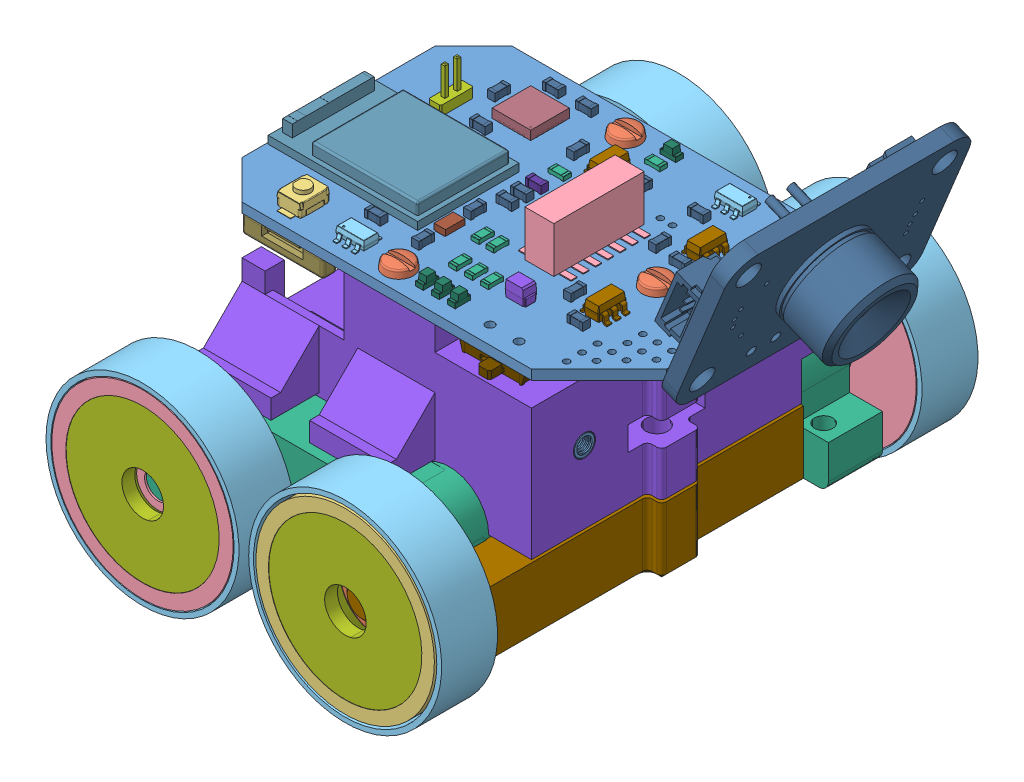
SolidWorks assembly AstroAnt_small_magnet, configuration Default. Lengths in mm.
Overall size (60.89 48.29 55.6).
184 component instances, 52 part files, 56 mates.
Components (placement in the parent):
- LiPo_360mAh-1: LiPo_360mAh [Default] at (6.0099 4.9998 47.0256) size (26.5 4.2 23.5) (hidden)
- 92120A150_Brass Heat-Set Inserts for Plastic-1: 92120A150_Brass Heat-Set Inserts for Plastic [92120A150] at (19.9543 12.4998 45.7029) size (2.56 3.33 2.56)
- 92120A150_Brass Heat-Set Inserts for Plastic-2: 92120A150_Brass Heat-Set Inserts for Plastic [92120A150] at (4.9543 12.4998 33.9529) size (2.56 3.33 2.56)
- 92120A150_Brass Heat-Set Inserts for Plastic-3: 92120A150_Brass Heat-Set Inserts for Plastic [92120A150] at (4.9543 12.4998 57.4529) size (2.56 3.33 2.56)
- 91460A005_METRIC CHEESE HEAD SLOTTED MACHINE SCREW-8: 91460A005_METRIC CHEESE HEAD SLOTTED MACHINE SCREW [91460A005] at (4.9543 14.9998 57.4529) x (1 0 0) z (0 1 0) size (3 3 7.1)
- 91460A005_METRIC CHEESE HEAD SLOTTED MACHINE SCREW-9: 91460A005_METRIC CHEESE HEAD SLOTTED MACHINE SCREW [91460A005] at (4.9543 14.9998 33.9529) x (1 0 0) z (0 1 0) size (3 3 7.1)
- 91460A005_METRIC CHEESE HEAD SLOTTED MACHINE SCREW-10: 91460A005_METRIC CHEESE HEAD SLOTTED MACHINE SCREW [91460A005] at (19.9543 14.9998 45.7029) x (1 0 0) z (0 1 0) size (3 3 7.1)
- 92120A150_Brass Heat-Set Inserts for Plastic-4: 92120A150_Brass Heat-Set Inserts for Plastic [92120A150] at (4.9543 -0.6002 57.4529) x (-0.616962 0 -0.786993) z (0.786993 0 -0.616962) size (2.56 3.33 2.56)
- 92120A150_Brass Heat-Set Inserts for Plastic-5: 92120A150_Brass Heat-Set Inserts for Plastic [92120A150] at (4.9543 -0.6002 33.9529) x (-0.616962 0 -0.786993) z (0.786993 0 -0.616962) size (2.56 3.33 2.56)
- mainboard_v1.step-1: mainboard_v1.step [Default] at (-103.0457 13.9998 235.7029) x (0 0 -1) z (0 1 0) size (29.41 41 10.8)
  - B3U-1000P.step-1: B3U-1000P.step [Default] at (178.95 -97.38 1.05) x (1 0 0) z (0 -1 0) size (4 1.75 2.5)
    - COMPOUND.step-1: COMPOUND.step [Default] at origin size (4 1.75 2.5)
  - 20021321-00014C1LF.step-1: 20021321-00014C1LF.step [Default] at (190 -115.5 1.05) size (9.35 5.45 4.85)
    - COMPOUND-0.step-1: COMPOUND-0.step [Default] at origin size (9.35 5.45 4.85)
  - MP6513GJ-Z.step-1: MP6513GJ-Z.step [Default] at (201.21 -120 1.05) x (-1 0 0) z (0 0 1) size (2.8 2.9 1)
    - COMPOUND-1.step-1: COMPOUND-1.step [Default] at origin size (2.8 2.9 1)
  - MP6513GJ-Z.step-2: MP6513GJ-Z.step [Default] at (178.51 -103.46 1.05) size (2.8 2.9 1)
    - COMPOUND-1.step-1: COMPOUND-1.step [Default] at origin size (2.8 2.9 1)
  - R_0603_1608Metric.step-1: R_0603_1608Metric.step [Default] at (195.55 -104.38 -0.05) x (1 0 0) z (0 0 -1) size (1.6 0.8 0.45)
    - SOLID.step-1: SOLID.step [Default] at origin size (1.6 0.8 0.45)
  - R_0603_1608Metric.step-2: R_0603_1608Metric.step [Default] at (192.6 -99.86 -0.05) x (0 1 0) z (0 0 -1) size (1.6 0.8 0.45)
    - SOLID.step-1: SOLID.step [Default] at origin size (1.6 0.8 0.45)
  - PinHeader_2x01_P1.27mm_Vertical.step-1: PinHeader_2x01_P1.27mm_Vertical.step [Default] at (194.96 -96.07 1.05) size (3.4 1.27 6.3)
    - SOLID-2.step-1: SOLID-2.step [Default] at origin size (3.4 1.27 6.3)
  - TAJP106K010RNJ.step-1: TAJP106K010RNJ.step [Default] at (196.22 -98.14 -0.05) x (-1 0 0) z (0 0 -1) size (2.05 1.4 1.7)
    - COMPOUND-3.step-1: COMPOUND-3.step [Default] at origin size (2.05 1.4 1.7)
  - TAJP106K010RNJ.step-2: TAJP106K010RNJ.step [Default] at (181.68 -117.23 1.05) x (0 1 0) z (0 0 1) size (2.05 1.4 1.7)
    - COMPOUND-3.step-1: COMPOUND-3.step [Default] at origin size (2.05 1.4 1.7)
  - SOT-23-5.step-1: SOT-23-5.step [Default] at (195.38 -122.78 1.05) x (0 1 0) z (0 0 1) size (2.8 2.9 1.55)
    - SOLID-4.step-1: SOLID-4.step [Default] at origin size (2.8 2.9 1.55)
  - C_0603_1608Metric.step-1: C_0603_1608Metric.step [Default] at (192.91 -122.55 1.05) x (0 -1 0) z (0 0 1) size (1.6 0.8 0.8)
    - SOLID-5.step-1: SOLID-5.step [Default] at origin size (1.6 0.8 0.8)
  - C_0603_1608Metric.step-2: C_0603_1608Metric.step [Default] at (193.57 -119.76 1.05) size (1.6 0.8 0.8)
    - SOLID-5.step-1: SOLID-5.step [Default] at origin size (1.6 0.8 0.8)
  - ECS-.327-12.5-12-TR.step-1: ECS-.327-12.5-12-TR.step [Default] at (184.31 -107.18 1.05) size (2 1.2 0.7)
    - COMPOUND-6.step-1: COMPOUND-6.step [Default] at origin size (2 1.2 0.7)
  - C_0603_1608Metric.step-3: C_0603_1608Metric.step [Default] at (197.67 -113.69 1.05) size (1.6 0.8 0.8)
    - SOLID-5.step-1: SOLID-5.step [Default] at origin size (1.6 0.8 0.8)
  - C_0603_1608Metric.step-4: C_0603_1608Metric.step [Default] at (197.64 -107.18 1.05) size (1.6 0.8 0.8)
    - SOLID-5.step-1: SOLID-5.step [Default] at origin size (1.6 0.8 0.8)
  - C_0603_1608Metric.step-5: C_0603_1608Metric.step [Default] at (190.96 -108.09 1.05) x (0 1 0) z (0 0 1) size (1.6 0.8 0.8)
    - SOLID-5.step-1: SOLID-5.step [Default] at origin size (1.6 0.8 0.8)
  - 1734592-6.step-1: 1734592-6.step [Default] at (203.79 -118 -1.05) x (0 -1 0) z (1 0 0) size (8.43 2.05 5.11)
    - SOLID-7.step-1: SOLID-7.step [Default] at origin size (8.43 2.05 5.11)
  - 1734592-6.step-2: 1734592-6.step [Default] at (176.19 -98 -1.05) x (0 1 0) z (-1 0 0) size (8.43 2.05 5.11)
    - SOLID-7.step-1: SOLID-7.step [Default] at origin size (8.43 2.05 5.11)
  - 20021321-00010C4LF.step-1: 20021321-00010C4LF.step [Default] at (190 -127.85 -0.05) x (1 0 0) z (0 0 -1) size (6.81 5.45 4.85)
    - COMPOUND-8.step-1: COMPOUND-8.step [Default] at origin size (6.81 5.45 4.85) (hidden)
  - 20021321-00010C4LF.step-2: 20021321-00010C4LF.step [Default] at (190 -127.85 1.05) size (6.81 5.45 4.85)
    - COMPOUND-8.step-1: COMPOUND-8.step [Default] at origin size (6.81 5.45 4.85) (hidden)
  - C_0603_1608Metric.step-6: C_0603_1608Metric.step [Default] at (181.31 -102.6 1.05) x (0 -1 0) z (0 0 1) size (1.6 0.8 0.8)
    - SOLID-5.step-1: SOLID-5.step [Default] at origin size (1.6 0.8 0.8)
  - C_0603_1608Metric.step-7: C_0603_1608Metric.step [Default] at (198.25 -119.14 1.05) x (0 -1 0) z (0 0 1) size (1.6 0.8 0.8)
    - SOLID-5.step-1: SOLID-5.step [Default] at origin size (1.6 0.8 0.8)
  - MPU6050.step-1: MPU6050.step [Default] at (198.43 -101.5 1.05) x (0 1 0) z (1 0 0) size (4 0.95 4)
    - COMPOUND-9.step-1: COMPOUND-9.step [Default] at origin size (4 0.95 4)
  - C_0603_1608Metric.step-8: C_0603_1608Metric.step [Default] at (194.9 -99.89 1.05) x (0 -1 0) z (0 0 1) size (1.6 0.8 0.8)
    - SOLID-5.step-1: SOLID-5.step [Default] at origin size (1.6 0.8 0.8)
  - C_0603_1608Metric.step-9: C_0603_1608Metric.step [Default] at (201.98 -100.38 1.05) x (0 -1 0) z (0 0 1) size (1.6 0.8 0.8)
    - SOLID-5.step-1: SOLID-5.step [Default] at origin size (1.6 0.8 0.8)
  - C_0603_1608Metric.step-10: C_0603_1608Metric.step [Default] at (201.98 -103.78 1.05) x (0 1 0) z (0 0 1) size (1.6 0.8 0.8)
    - SOLID-5.step-1: SOLID-5.step [Default] at origin size (1.6 0.8 0.8)
  - C_0603_1608Metric.step-11: C_0603_1608Metric.step [Default] at (198.81 -97.82 1.05) size (1.6 0.8 0.8)
    - SOLID-5.step-1: SOLID-5.step [Default] at origin size (1.6 0.8 0.8)
  - SOT-23-5.step-2: SOT-23-5.step [Default] at (184.86 -122.77 1.05) x (0 1 0) z (0 0 1) size (2.8 2.9 1.55)
    - SOLID-4.step-1: SOLID-4.step [Default] at origin size (2.8 2.9 1.55)
  - SOT-23-5.step-3: SOT-23-5.step [Default] at (197.58 -110.46 1.05) x (0 1 0) z (0 0 1) size (2.8 2.9 1.55)
    - SOLID-4.step-1: SOLID-4.step [Default] at origin size (2.8 2.9 1.55)
  - MDBT50Q-1MV2.step-1: MDBT50Q-1MV2.step [Default] at (187.3136 -98.605 1.0754) x (-1 0 0) z (0 1 0) size (10.5 2.06 15.5)
    - SOLID-10.step-1: SOLID-10.step [Default] at origin size (10.5 2.06 15.5)
  - C_0603_1608Metric.step-12: C_0603_1608Metric.step [Default] at (189.44 -108.09 1.05) x (0 1 0) z (0 0 1) size (1.6 0.8 0.8)
    - SOLID-5.step-1: SOLID-5.step [Default] at origin size (1.6 0.8 0.8)
  - C_0603_1608Metric.step-13: C_0603_1608Metric.step [Default] at (181.57 -107.18 1.05) x (-1 0 0) z (0 0 1) size (1.6 0.8 0.8)
    - SOLID-5.step-1: SOLID-5.step [Default] at origin size (1.6 0.8 0.8)
  - C_0603_1608Metric.step-14: C_0603_1608Metric.step [Default] at (186.97 -107.18 1.05) size (1.6 0.8 0.8)
    - SOLID-5.step-1: SOLID-5.step [Default] at origin size (1.6 0.8 0.8)
  - C_0603_1608Metric.step-15: C_0603_1608Metric.step [Default] at (184.77 -119.75 1.05) x (-1 0 0) z (0 0 1) size (1.6 0.8 0.8)
    - SOLID-5.step-1: SOLID-5.step [Default] at origin size (1.6 0.8 0.8)
  - C_0603_1608Metric.step-16: C_0603_1608Metric.step [Default] at (182.37 -122.54 1.05) x (0 -1 0) z (0 0 1) size (1.6 0.8 0.8)
    - SOLID-5.step-1: SOLID-5.step [Default] at origin size (1.6 0.8 0.8)
  - LED_0603_1608Metric.step-1: LED_0603_1608Metric.step [Default] at (178.19 -111.01 1.05) size (1.6 0.8 1.1)
    - SOLID-11.step-1: SOLID-11.step [Default] at origin size (1.6 0.8 1.1)
  - LED_0603_1608Metric.step-2: LED_0603_1608Metric.step [Default] at (178.19 -112.66 1.05) size (1.6 0.8 1.1)
    - SOLID-11.step-1: SOLID-11.step [Default] at origin size (1.6 0.8 1.1)
  - LED_0603_1608Metric.step-3: LED_0603_1608Metric.step [Default] at (178.19 -114.31 1.05) size (1.6 0.8 1.1)
    - SOLID-11.step-1: SOLID-11.step [Default] at origin size (1.6 0.8 1.1)
  - LED_0603_1608Metric.step-4: LED_0603_1608Metric.step [Default] at (202.34 -112.21 1.05) x (0 1 0) z (0 0 1) size (1.6 0.8 1.1)
    - SOLID-11.step-1: SOLID-11.step [Default] at origin size (1.6 0.8 1.1)
  - 473460001.step-1: 473460001.step [Default] at (201.68 -99.72 -1.25) x (0 -1 0) z (1 0 0) size (7.98 2.94 5.43)
    - COMPOUND-12.step-1: COMPOUND-12.step [Default] at origin size (7.98 2.94 5.43)
  - L_0603_1608Metric.step-1: L_0603_1608Metric.step [Default] at (192.48 -108.09 1.05) x (0 1 0) z (0 0 1) size (1.6 0.8 0.8)
    - SOLID-13.step-1: SOLID-13.step [Default] at origin size (1.6 0.8 0.8)
  - R_0603_1608Metric.step-3: R_0603_1608Metric.step [Default] at (185.18 -111.31 1.05) x (-1 0 0) z (0 0 1) size (1.6 0.8 0.45)
    - SOLID.step-1: SOLID.step [Default] at origin size (1.6 0.8 0.45)
  - R_0603_1608Metric.step-4: R_0603_1608Metric.step [Default] at (185.18 -109.77 1.05) size (1.6 0.8 0.45)
    - SOLID.step-1: SOLID.step [Default] at origin size (1.6 0.8 0.45)
  - R_0603_1608Metric.step-5: R_0603_1608Metric.step [Default] at (181.62 -111.01 1.05) size (1.6 0.8 0.45)
    - SOLID.step-1: SOLID.step [Default] at origin size (1.6 0.8 0.45)
  - R_0603_1608Metric.step-6: R_0603_1608Metric.step [Default] at (181.62 -112.66 1.05) size (1.6 0.8 0.45)
    - SOLID.step-1: SOLID.step [Default] at origin size (1.6 0.8 0.45)
  - R_0603_1608Metric.step-7: R_0603_1608Metric.step [Default] at (181.62 -114.31 1.05) x (-1 0 0) z (0 0 1) size (1.6 0.8 0.45)
    - SOLID.step-1: SOLID.step [Default] at origin size (1.6 0.8 0.45)
  - R_0603_1608Metric.step-8: R_0603_1608Metric.step [Default] at (194.84 -108.1 1.05) x (0 1 0) z (0 0 1) size (1.6 0.8 0.45)
    - SOLID.step-1: SOLID.step [Default] at origin size (1.6 0.8 0.45)
  - R_0603_1608Metric.step-9: R_0603_1608Metric.step [Default] at (200.69 -112.2325 1.05) x (0 1 0) z (0 0 1) size (1.6 0.8 0.45)
    - SOLID.step-1: SOLID.step [Default] at origin size (1.6 0.8 0.45)
  - R_0603_1608Metric.step-10: R_0603_1608Metric.step [Default] at (196.22 -101.51 -0.05) x (-1 0 0) z (0 0 -1) size (1.6 0.8 0.45)
    - SOLID.step-1: SOLID.step [Default] at origin size (1.6 0.8 0.45)
  - R_0603_1608Metric.step-11: R_0603_1608Metric.step [Default] at (196.22 -99.9725 -0.05) x (-1 0 0) z (0 0 -1) size (1.6 0.8 0.45)
    - SOLID.step-1: SOLID.step [Default] at origin size (1.6 0.8 0.45)
  - SW_SPDT_PCM12.step-1: SW_SPDT_PCM12.step [Default] at (178.18 -119.37 -0.05) x (0 1 0) z (0 0 -1) size (7.7 5 2)
    - SOLID-14.step-1: SOLID-14.step [Default] at origin size (7.7 5 2)
  - COMPOUND-15.step-1: COMPOUND-15.step [Default] at origin size (28 41 1)
- ball_bearing_5x11x4mm-1: ball_bearing_5x11x4mm [Default] at (-65.9801 -4.7758 21.2029) x (0.999925 -0.012245 0) z (0 0 1) size (8 8 2.5)
- wheel_holder_non_motor-1: wheel_holder_non_motor [Default] at (-90.7699 -0.8362 17.9029) size (18.5 18.5 5.8)
- wheel_holder_non_motor-2: wheel_holder_non_motor [Default] at (1.3792 -86.6559 73.5029) x (0.185441 0.982655 0) z (0 0 -1) size (18.5 18.5 5.8)
- ball_bearing_5x11x4mm-2: ball_bearing_5x11x4mm [Default] at (-9.788 -57.5376 70.2029) x (0.373101 0.927791 0) z (0 0 -1) size (8 8 2.5)
- wheel_motor-1: wheel_motor [Default] at (44.5289 -0.8963 17.9029) size (18.8 18.8 5.8)
- wheel_motor-2: wheel_motor [Default] at (-4.9746 26.526 73.5029) x (-0.038296 0.999266 0) z (0 0 -1) size (18.8 18.8 5.8)
- tire-1: tire [Default] at (58.6593 -4.042 17.9029) size (20 20 5.8)
- tire-2: tire [Default] at (37.6493 -4.042 17.9029) size (20 20 5.8)
- tire-3: tire [Default] at (58.6593 -4.042 67.7029) size (20 20 5.8)
- tire-4: tire [Default] at (37.6493 -4.042 67.7029) size (20 20 5.8)
- PA2-50_with_gearbox-3: PA2-50_with_gearbox [Default] at (45.51 -3.6027 60.1029) x (-1 0 0) z (0 0 1) size (30.92 12.52 38.5)
  - PA2-50-1: PA2-50 [Default] at (26.117 -19.7771 -19.1) x (0 0 1) z (0.954024 0.299729 0) size (29.1 8 8) (hidden)
  - gearbox-1: gearbox [Default] at origin size (29.9 11.5 13.6)
- PA2-50_with_gearbox-4: PA2-50_with_gearbox [Default] at (-35.6268 -3.6027 31.3029) x (1 0 0) z (0 0 -1) size (30.92 12.52 38.5)
  - PA2-50-1: PA2-50 [Default] at (26.117 -19.7771 -19.1) x (0 0 1) z (0.954024 0.299729 0) size (29.1 8 8) (hidden)
  - gearbox-1: gearbox [Default] at origin size (29.9 11.5 13.6)
- RA22CS-N-1: RA22CS-N [Default] at (15.4466 -2.6002 19.5154) x (1 0 0) z (0 -1 0) size (15.88 3.17 15.88)
- RA22CS-N-2: RA22CS-N [Default] at (-5.5634 -2.6002 19.5154) x (1 0 0) z (0 -1 0) size (15.88 3.17 15.88)
- RA22CS-N-3: RA22CS-N [Default] at (-5.5634 -2.6002 71.8904) x (-0.968047 -0.250767 0) z (0.250767 -0.968047 0) size (15.88 3.17 15.88)
- RA22CS-N-4: RA22CS-N [Default] at (15.4466 -2.6002 71.8904) x (-0.968047 -0.250767 0) z (0.250767 -0.968047 0) size (15.88 3.17 15.88)
- robobody-1: robobody [Default] at (-9.0457 6.9406 -0.9986) size (31.5 16.1 38)
- 92120A150_Brass Heat-Set Inserts for Plastic-6: 92120A150_Brass Heat-Set Inserts for Plastic [92120A150] at (19.9543 -0.6002 45.7029) x (-0.616962 0 -0.786993) z (0.786993 0 -0.616962) size (2.56 3.33 2.56)
- motor_holder_2-1: motor_holder_2 [Default] at (52.4112 -9.4002 -5.2676) size (31.5 8.8 52.2)
- 92120A150_Brass Heat-Set Inserts for Plastic-7: 92120A150_Brass Heat-Set Inserts for Plastic [92120A150] at (19.4543 5.3998 54.2029) x (0 1 0) z (0 0 1) size (2.56 3.33 2.56)
- 92120A150_Brass Heat-Set Inserts for Plastic-8: 92120A150_Brass Heat-Set Inserts for Plastic [92120A150] at (19.4543 5.3998 37.2029) x (0 1 0) z (0 0 1) size (2.56 3.33 2.56)
- impedance_measurement2-impedance_measurement.step-1: impedance_measurement2-impedance_measurement.step [Default] at (27.9543 22.4998 52.7029) x (0 0 -1) z (0 1 0) size (24 25 7.6) (hidden)
  - Board_Geoms_58a9.step-1: Board_Geoms_58a9.step [Default] at origin size (24 25 1.65)
    - Pcb_58a9.step-1: Pcb_58a9.step [Default] at (-125 125 0) size (24 25 1.6)
    - topPads_58a9.step-1: topPads_58a9.step [Default] at (-125 125 0.02) size (21.67 21.95 0.01)
    - topTracks_58a9.step-1: topTracks_58a9.step [Default] at (-125 125 0.01) size (22.19 20.2 0.01)
    - topZones_58a9.step-1: topZones_58a9.step [Default] at (-125 125 0.01) size (1.81 1.01 0.01)
    - botPads_58a9.step-1: botPads_58a9.step [Default] at (-125 125 -1.62) size (20.66 21.93 0.01)
    - botTracks_58a9.step-1: botTracks_58a9.step [Default] at (-125 125 -1.61) size (19.15 19.69 0.01)
    - botZones_58a9.step-1: botZones_58a9.step [Default] at (-125 125 -1.61)
  - Step_Models_58a9.step-1: Step_Models_58a9.step [Default] at origin size (21.21 18.41 7.6)
    - Top_58a9.step-1: Top_58a9.step [Default] at origin size (21.21 14.13 2)
      - U1_ASSEMBLY_616EAA5E.step-1: U1_ASSEMBLY_616EAA5E.step [Default] at (13.84 11.34 0) size (6 4.9 1.75)
        - Body.step-1: Body.step [Default] at origin size (3.9 4.9 1.57)
        - PinsArrayLR.step-1: PinsArrayLR.step [Default] at origin size (6 4.22 1)
      - U2_ASSEMBLY_6195A977.step-1: U2_ASSEMBLY_6195A977.step [Default] at (0.61 8.84 0) x (-1 0 0) z (0 0 1) size (7.8 6.2 2)
        - Body001.step-1: Body001.step [Default] at origin size (5.3 6.2 1.95)
        - PinsArrayLR001.step-1: PinsArrayLR001.step [Default] at origin size (7.8 4.85 1.09)
      - C9_C_0603_1608Metric_6195A5CF.step-1: C9_C_0603_1608Metric_6195A5CF.step [Default] at (7.13 19.31 0) size (1.6 0.8 0.8)
      - R11_R_0805_2012Metric_6195A804.step-1: R11_R_0805_2012Metric_6195A804.step [Default] at (14.1 18.66 0) size (2 1.2 0.45)
      - C9_C_0603_1608Metric_6195A5CF.step-2: C9_C_0603_1608Metric_6195A5CF.step [Default] at (16.32 15.88 0) x (0 -1 0) z (0 0 1) size (1.6 0.8 0.8)
      - R10_R_0402_1005Metric_inf.step-1: R10_R_0402_1005Metric_inf.step [Default] at (7.27 8.57 0) x (0 1 0) z (0 0 1) size (1 0.5 0.35)
      - R10_R_0402_1005Metric_inf.step-2: R10_R_0402_1005Metric_inf.step [Default] at (6.06 8.57 0) x (0 1 0) z (0 0 1) size (1 0.5 0.35)
      - R10_R_0402_1005Metric_inf.step-3: R10_R_0402_1005Metric_inf.step [Default] at (9.01 9.43 0) x (-1 0 0) z (0 0 1) size (1 0.5 0.35)
      - R10_R_0402_1005Metric_inf.step-4: R10_R_0402_1005Metric_inf.step [Default] at (7.06 11.59 0) x (-1 0 0) z (0 0 1) size (1 0.5 0.35)
      - R10_R_0402_1005Metric_inf.step-5: R10_R_0402_1005Metric_inf.step [Default] at (15.52 7.36 0) x (0 1 0) z (0 0 1) size (1 0.5 0.35)
      - R10_R_0402_1005Metric_inf.step-6: R10_R_0402_1005Metric_inf.step [Default] at (16.82 7.36 0) x (0 -1 0) z (0 0 1) size (1 0.5 0.35)
      - C5_C_0402_1005Metric_616E5CDC.step-1: C5_C_0402_1005Metric_616E5CDC.step [Default] at (7.09 10.42 0) x (-1 0 0) z (0 0 1) size (1 0.5 0.5)
      - U3_TSOT_23_5_616E36B3.step-1: U3_TSOT_23_5_616E36B3.step [Default] at (0.38 16.55 0) x (0 -1 0) z (0 0 1) size (2.8 2.9 0.95)
      - R8_R_0603_1608Metric_inf.step-1: R8_R_0603_1608Metric_inf.step [Default] at (9.74 6.91 0) x (-1 0 0) z (0 0 1) size (1.6 0.8 0.45)
      - C9_C_0603_1608Metric_6195A5CF.step-3: C9_C_0603_1608Metric_6195A5CF.step [Default] at (-2.15 17 0) x (0 1 0) z (0 0 1) size (1.6 0.8 0.8)
      - C9_C_0603_1608Metric_6195A5CF.step-4: C9_C_0603_1608Metric_6195A5CF.step [Default] at (0.46 13.71 0) size (1.6 0.8 0.8)
      - C9_C_0603_1608Metric_6195A5CF.step-5: C9_C_0603_1608Metric_6195A5CF.step [Default] at (-1.47 19.47 0) size (1.6 0.8 0.8)
      - C9_C_0603_1608Metric_6195A5CF.step-6: C9_C_0603_1608Metric_6195A5CF.step [Default] at (-2.96 12.84 0) size (1.6 0.8 0.8)
      - C9_C_0603_1608Metric_6195A5CF.step-7: C9_C_0603_1608Metric_6195A5CF.step [Default] at (-3.74 17.02 0) x (0 -1 0) z (0 0 1) size (1.6 0.8 0.8)
      - C9_C_0603_1608Metric_6195A5CF.step-8: C9_C_0603_1608Metric_6195A5CF.step [Default] at (-2.96 14.45 0) x (-1 0 0) z (0 0 1) size (1.6 0.8 0.8)
    - Bot_58a9.step-1: Bot_58a9.step [Default] at origin size (14.64 18.41 6.3)
      - R10_R_0402_1005Metric_inf.step-1: R10_R_0402_1005Metric_inf.step [Default] at (-2.7 9.16 -1.6) x (-1 0 0) z (0 0 -1) size (1 0.5 0.35)
      - R10_R_0402_1005Metric_inf.step-2: R10_R_0402_1005Metric_inf.step [Default] at (3.08 7.15 -1.6) x (1 0 0) z (0 0 -1) size (1 0.5 0.35)
      - R10_R_0402_1005Metric_inf.step-3: R10_R_0402_1005Metric_inf.step [Default] at (1.08 9.94 -1.6) x (-0.707107 -0.707107 0) z (0 0 -1) size (1 0.5 0.35)
      - J4_PinHeader_2x05_P127mm_Vertical_616E426E.step-1: J4_PinHeader_2x05_P127mm_Vertical_616E426E.step [Default] at (4.46 3.83 -1.6) x (0 -1 0) z (0 0 -1) size (3.4 6.35 6.3)
      - J3_PinHeader_2x07_P127mm_Vertical_616E4D18.step-1: J3_PinHeader_2x07_P127mm_Vertical_616E4D18.step [Default] at (3.19 16.45 -1.6) x (0 -1 0) z (0 0 -1) size (3.4 8.89 6.3)
      - C9_C_0603_1608Metric_6195A5CF.step-1: C9_C_0603_1608Metric_6195A5CF.step [Default] at (2.85 19.51 -1.6) x (-1 0 0) z (0 0 -1) size (1.6 0.8 0.8)
- 9mm_pogo_pin-1: 9mm_pogo_pin [Default] at (4.8543 -7.1002 37.7029) x (0.948575 0 -0.316551) z (0.316551 0 0.948575) size (2 9 2) (hidden)
- 9mm_pogo_pin-2: 9mm_pogo_pin [Default] at (4.8543 -7.1002 53.7029) x (0.905311 0 -0.424749) z (0.424749 0 0.905311) size (2 9 2) (hidden)
- MLX90640-1: MLX90640 [默认] at (33.2982 16.1667 32.4384) x (0 0 1) z (-0.925385 0.379028 0) size (25.4 17.78 11.7)
- IR_camera_holder-1: IR_camera_holder [默认] at origin
Mates (geometry in assembly coordinates):
- Concentric63: concentric anti-aligned: cylinder of ball_bearing_5x11x4mm-1 through (-5.5634 -2.6002 23.7029) axis (0 0 -1) radius 4; cylinder of wheel_holder_non_motor-1 through (-5.5634 -2.6002 17.9029) axis (0 0 1) radius 4
- Coincident105: coincident aligned: plane of ball_bearing_5x11x4mm-1 through (-5.5634 -2.6002 23.7029) normal (0 0 1); plane of wheel_holder_non_motor-1 through (-5.5634 -2.6002 23.7029) normal (0 0 1)
- Coincident107: coincident aligned: plane of wheel_holder_non_motor-2 through (15.4466 -2.6002 67.7029) normal (0 0 -1); plane of ball_bearing_5x11x4mm-2 through (15.4466 -2.6002 67.7029) normal (0 0 -1)
- Concentric83: concentric anti-aligned: cylinder of wheel_motor-1 through (15.4466 -2.6002 23.7029) axis (0 0 -1) radius 9.4; cylinder of tire-1 through (15.4466 -2.6002 17.9029) axis (0 0 1) radius 9.5
- Coincident123: coincident aligned: plane of wheel_motor-1 through (15.4466 -2.6002 17.9029) normal (0 0 -1); plane of tire-1 through (15.4466 -2.6002 17.9029) normal (0 0 -1)
- Concentric84: concentric anti-aligned: cylinder of wheel_holder_non_motor-1 through (-5.5634 -2.6002 23.7029) axis (0 0 -1) radius 9.25; cylinder of tire-2 through (-5.5634 -2.6002 17.9029) axis (0 0 1) radius 9.5
- Coincident124: coincident aligned: plane of wheel_holder_non_motor-1 through (-5.5634 -2.6002 17.9029) normal (0 0 -1); plane of tire-2 through (-5.5634 -2.6002 17.9029) normal (0 0 -1)
- Coincident125: coincident aligned: plane of wheel_motor-2 through (-5.5634 -2.6002 73.5029) normal (0 0 1); plane of tire-4 through (-5.5634 -2.6002 73.5029) normal (0 0 1)
- Concentric85: concentric aligned: cylinder of wheel_motor-2 through (-5.5634 -2.6002 67.7029) axis (0 0 1) radius 9.4; cylinder of tire-4 through (-5.5634 -2.6002 67.7029) axis (0 0 1) radius 9.5
- Coincident126: coincident aligned: plane of wheel_holder_non_motor-2 through (15.4466 -2.6002 73.5029) normal (0 0 1); plane of tire-3 through (15.4466 -2.6002 73.5029) normal (0 0 1)
- Concentric86: concentric aligned: cylinder of wheel_holder_non_motor-2 through (15.4466 -2.6002 67.7029) axis (0 0 1) radius 9.25; cylinder of tire-3 through (15.4466 -2.6002 67.7029) axis (0 0 1) radius 9.5
- Concentric100: concentric anti-aligned: cylinder of wheel_holder_non_motor-2 through (15.4466 -2.6002 73.5029) axis (0 0 -1) radius 4; cylinder of ball_bearing_5x11x4mm-2 through (15.4466 -2.6002 66.2029) axis (0 0 1) radius 2
- Coincident138: coincident aligned: plane of wheel_holder_non_motor-2 through (15.4466 -2.6002 67.7029) normal (0 0 -1); plane of ball_bearing_5x11x4mm-2 through (15.4466 -2.6002 67.7029) normal (0 0 -1)
- Concentric110: concentric anti-aligned: cylinder of wheel_motor-2 through (-5.5634 -2.6002 67.7029) axis (0 0 1) radius 1.4; cylinder of PA2-50_with_gearbox-3/gearbox-1 through (-5.5634 -2.6002 71.7029) axis (0 0 -1) radius 1.45
- Concentric111: concentric aligned: cylinder of tire-1 through (15.4466 -2.6002 23.7029) axis (0 0 -1) radius 10; cylinder of tire-3 through (15.4466 -2.6002 73.5029) axis (0 0 -1) radius 10
- Concentric112: concentric aligned: cylinder of tire-2 through (-5.5634 -2.6002 23.7029) axis (0 0 -1) radius 10; cylinder of tire-4 through (-5.5634 -2.6002 73.5029) axis (0 0 -1) radius 10
- Coincident144: coincident aligned: plane of PA2-50_with_gearbox-3/gearbox-1 through (16.4366 -9.1002 65.7029) normal (0 -1 0); plane of PA2-50_with_gearbox-4/gearbox-1 through (-6.5534 -9.1002 25.7029) normal (0 -1 0)
- Coincident145: coincident aligned: plane of wheel_holder_non_motor-1 through (-5.5634 -2.6002 17.9029) normal (0 0 -1); plane of wheel_motor-1 through (15.4466 -2.6002 17.9029) normal (0 0 -1)
- Coincident146: coincident aligned: plane of wheel_holder_non_motor-2 through (15.4466 -2.6002 73.5029) normal (0 0 1); plane of wheel_motor-2 through (-5.5634 -2.6002 73.5029) normal (0 0 1)
- Coincident149: coincident anti-aligned: plane of wheel_motor-1 through (15.4466 -2.6002 21.1029) normal (0 0 -1); plane of RA22CS-N-1 through (15.4466 -2.6002 21.1029) normal (0 0 1)
- Concentric113: concentric aligned: cylinder of wheel_motor-1 through (15.4466 -2.6002 23.7029) axis (0 0 -1) radius 1.4; cylinder of RA22CS-N-1 through (15.4466 -2.6002 19.5154) axis (0 0 -1) radius 2.159
- Concentric114: concentric aligned: cylinder of wheel_holder_non_motor-1 through (-5.5634 -2.6002 21.1029) axis (0 0 -1) radius 7.95; cylinder of RA22CS-N-2 through (-5.5634 -2.6002 19.5154) axis (0 0 -1) radius 2.159
- Coincident150: coincident anti-aligned: plane of wheel_holder_non_motor-1 through (-5.5634 -2.6002 21.1029) normal (0 0 -1); plane of RA22CS-N-2 through (-5.5634 -2.6002 21.1029) normal (0 0 1)
- Concentric115: concentric aligned: cylinder of wheel_motor-2 through (-5.5634 -2.6002 70.3029) axis (0 0 1) radius 7.95; cylinder of RA22CS-N-3 through (-5.5634 -2.6002 70.3029) axis (0 0 1) radius 7.9375
- Coincident151: coincident anti-aligned: plane of wheel_motor-2 through (-5.5634 -2.6002 70.3029) normal (0 0 1); plane of RA22CS-N-3 through (-5.5634 -2.6002 70.3029) normal (0 0 -1)
- Concentric116: concentric aligned: cylinder of wheel_holder_non_motor-2 through (15.4466 -2.6002 70.3029) axis (0 0 1) radius 7.95; cylinder of RA22CS-N-4 through (15.4466 -2.6002 70.3029) axis (0 0 1) radius 7.9375
- Coincident152: coincident anti-aligned: plane of wheel_holder_non_motor-2 through (15.4466 -2.6002 70.3029) normal (0 0 1); plane of RA22CS-N-4 through (15.4466 -2.6002 70.3029) normal (0 0 -1)
- Coincident153: coincident aligned: plane of mainboard_v1.step-1/COMPOUND-15.step-1 through (20.9543 13.9998 59.7029) normal (0 0 1); plane of robobody-1 through (20.9543 13.9998 59.7029) normal (0 0 1)
- Coincident154: coincident: line of mainboard_v1.step-1/COMPOUND-15.step-1 through (-9.0457 13.9998 59.7029) axis (0 1 0); plane of robobody-1 through (-9.0457 6.9406 -0.9986) normal (-1 0 0)
- Concentric121: concentric aligned: cylinder of 92120A150_Brass Heat-Set Inserts for Plastic-4 through (4.9543 0.8998 57.4529) axis (0 1 0) radius 1.075; cylinder of robobody-1 through (4.9543 -2.1591 57.4529) axis (0 1 0) radius 1.15
- Concentric122: concentric aligned: cylinder of 92120A150_Brass Heat-Set Inserts for Plastic-5 through (4.9543 0.8998 33.9529) axis (0 1 0) radius 1.075; cylinder of robobody-1 through (4.9543 -2.1591 33.9529) axis (0 1 0) radius 1.15
- Concentric123: concentric aligned: cylinder of robobody-1 through (19.9543 -2.1591 45.7029) axis (0 1 0) radius 1.15; cylinder of 92120A150_Brass Heat-Set Inserts for Plastic-6 through (19.9543 0.8998 45.7029) axis (0 1 0) radius 1.075
- Coincident164: coincident anti-aligned: plane of PA2-50_with_gearbox-4/gearbox-1 through (12.2966 -5.4002 30.3029) normal (0 -1 0); plane of motor_holder_2-1 through (-9.0457 -5.4002 31.5029) normal (0 1 0)
- Coincident167: coincident aligned: plane of robobody-1 through (20.9543 6.9406 -0.9986) normal (1 0 0); plane of motor_holder_2-1 through (20.9543 -2.4002 61.1029) normal (1 0 0)
- Concentric124: concentric anti-aligned: cylinder of PA2-50_with_gearbox-3/PA2-50-1 through (12.4366 -2.1002 57.2029) axis (0 0 -1) radius 4; cylinder of robobody-1 through (12.4366 -2.1002 32.5029) axis (0 0 1) radius 4.1
- Concentric125: concentric anti-aligned: cylinder of PA2-50_with_gearbox-4/PA2-50-1 through (-2.5534 -2.1002 34.2029) axis (0 0 1) radius 4; cylinder of robobody-1 through (-2.5534 -2.1002 58.9029) axis (0 0 -1) radius 4.1
- Coincident174: coincident anti-aligned: plane of PA2-50_with_gearbox-4/gearbox-1 through (-2.5534 -2.1002 31.7029) normal (0 0 1); plane of robobody-1 through (20.9543 13.9998 31.7029) normal (0 0 -1)
- Coincident175: coincident anti-aligned: plane of PA2-50_with_gearbox-3/gearbox-1 through (12.4366 -2.1002 59.7029) normal (0 0 -1); plane of robobody-1 through (20.9543 13.9998 59.7029) normal (0 0 1)
- Coincident176: coincident anti-aligned: plane of mainboard_v1.step-1/COMPOUND-15.step-1 through (6.7692 13.9998 45.7029) normal (0 -1 0); plane of robobody-1 through (20.9543 13.9998 59.7029) normal (0 1 0)
- Concentric126: concentric anti-aligned: cylinder of robobody-1 through (14.5016 5.3998 54.2029) axis (1 0 0) radius 1.15; cylinder of 92120A150_Brass Heat-Set Inserts for Plastic-7 through (17.9543 5.3998 54.2029) axis (-1 0 0) radius 1.075
- Concentric127: concentric anti-aligned: cylinder of robobody-1 through (14.5016 5.3998 37.2029) axis (1 0 0) radius 1.15; cylinder of 92120A150_Brass Heat-Set Inserts for Plastic-8 through (17.9543 5.3998 37.2029) axis (-1 0 0) radius 1.075
- Coincident177: coincident aligned: plane of robobody-1 through (20.9543 6.9406 -0.9986) normal (1 0 0); plane of 92120A150_Brass Heat-Set Inserts for Plastic-8 through (20.9543 4.5998 37.2029) normal (1 0 0)
- Coincident178: coincident aligned: plane of robobody-1 through (20.9543 6.9406 -0.9986) normal (1 0 0); plane of 92120A150_Brass Heat-Set Inserts for Plastic-7 through (20.9543 4.5998 54.2029) normal (1 0 0)
- Distance1: distance = 2 mm anti-aligned: plane of wheel_motor-2 through (-5.5634 -2.6002 67.7029) normal (0 0 -1); plane of PA2-50_with_gearbox-3/gearbox-1 through (45.51 -3.6027 65.7029) normal (0 0 1)
- Distance2: distance = 2 mm anti-aligned: plane of wheel_motor-1 through (15.4466 -2.6002 23.7029) normal (0 0 1); plane of PA2-50_with_gearbox-4/gearbox-1 through (-35.6268 -3.6027 25.7029) normal (0 0 -1)
- Concentric128: concentric anti-aligned: cylinder of PA2-50_with_gearbox-4/gearbox-1 through (15.4466 -2.6002 19.7029) axis (0 0 1) radius 1.45; cylinder of RA22CS-N-1 through (15.4466 -2.6002 19.5154) axis (0 0 -1) radius 2.159
- Distance9: distance = 0.25 mm anti-aligned: plane of LiPo_360mAh-1 through (15.7543 9.1998 57.4529) normal (0 0 1); plane of robobody-1 through (42.4929 9.9998 57.7029) normal (0 0 -1)
- Coincident222: coincident anti-aligned: plane of LiPo_360mAh-1 through (17.7543 4.9998 47.0256) normal (1 0 0); plane of robobody-1 through (17.7543 3.9998 36.2029) normal (-1 0 0)
- Coincident223: coincident anti-aligned: plane of mainboard_v1.step-1/20021321-00010C4LF.step-2/COMPOUND-8.step-1 through (24.8043 19.8998 45.7029) normal (0 1 0); plane of impedance_measurement2-impedance_measurement.step-1/Step_Models_58a9.step-1/Bot_58a9.step-1/J4_PinHeader_2x05_P127mm_Vertical_616E426E.step-1 through (24.7593 19.8998 45.7029) normal (0 -1 0)
- Coincident224: coincident aligned: plane of mainboard_v1.step-1/COMPOUND-15.step-1 through (27.9543 13.9998 38.7029) normal (1 0 0); plane of impedance_measurement2-impedance_measurement.step-1/Board_Geoms_58a9.step-1/Pcb_58a9.step-1 through (27.9543 22.4998 38.7029) normal (1 0 0)
- Distance10: distance = 0.23 mm aligned: plane of impedance_measurement2-impedance_measurement.step-1/Step_Models_58a9.step-1/Bot_58a9.step-1/J4_PinHeader_2x05_P127mm_Vertical_616E426E.step-1 through (23.1863 20.8998 42.5279) normal (0 0 -1); plane of mainboard_v1.step-1/20021321-00010C4LF.step-2/COMPOUND-8.step-1 through (23.3043 15.1498 42.2979) normal (0 0 -1)
- Concentric129: concentric anti-aligned: cylinder of robobody-1 through (4.8543 -7.2616 53.7029) axis (0 -1 0) radius 1.5; cylinder of 9mm_pogo_pin-2 through (4.8543 -11.6002 53.7029) axis (0 1 0) radius 0.75
- Concentric130: concentric anti-aligned: cylinder of robobody-1 through (4.8543 -7.2616 37.7029) axis (0 -1 0) radius 1.5; cylinder of 9mm_pogo_pin-1 through (4.8543 -11.6002 37.7029) axis (0 1 0) radius 0.75
- Distance11: distance = 4.2 mm aligned: plane of 9mm_pogo_pin-2 through (4.8543 -13.6002 53.7029) normal (0 -1 0); plane of motor_holder_2-1 through (52.4112 -9.4002 -5.2676) normal (0 -1 0)
- Distance12: distance = 4.2 mm aligned: plane of 9mm_pogo_pin-1 through (4.8543 -13.6002 37.7029) normal (0 -1 0); plane of motor_holder_2-1 through (52.4112 -9.4002 -5.2676) normal (0 -1 0)
- Parallel1: parallel aligned: plane of robobody-1 through (20.9543 13.9998 59.7029) normal (0 0 1); plane of MLX90640-1 through (34.2609 18.5172 57.8384) normal (0 0 1)
